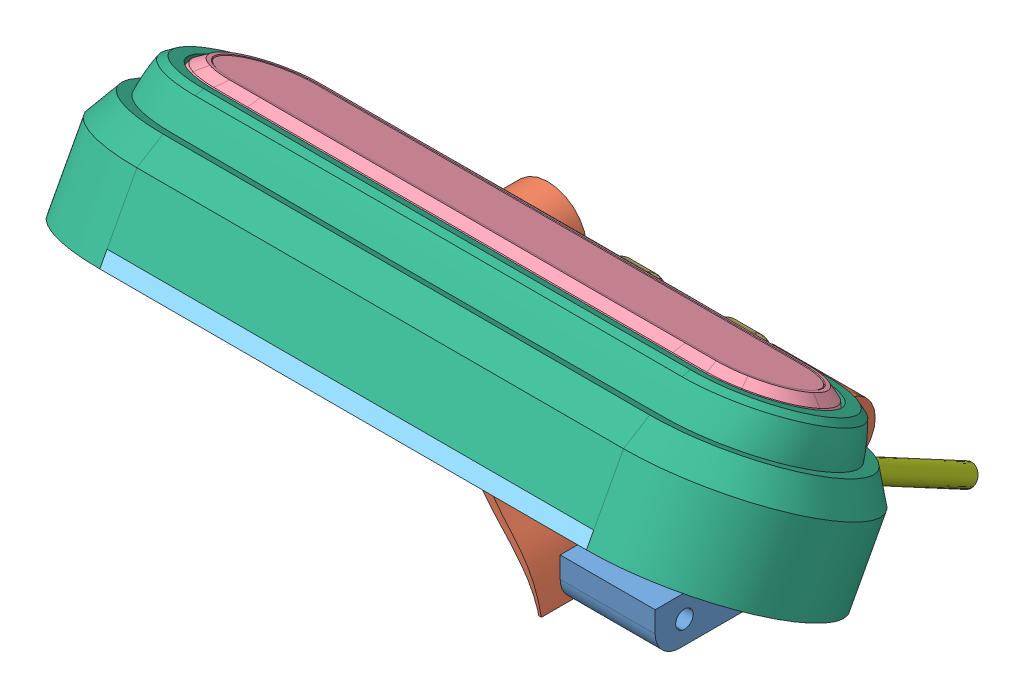
SolidWorks assembly realsense_mount, configuration Default. Lengths in mm.
Overall size (141.5 99.34 86.29).
8 component instances, 7 part files, 15 mates.
Components (placement in the parent):
- camera_mount_clamp-1: camera_mount_clamp [Default] at (0 -14.2875 0) x (0 0 1) z (-1 0 0)
- bike_clamp_pin-1: bike_clamp_pin [Default] at (1.038 25.4 0) x (0 1 0) z (0 0 1)
- camera_support-1: camera_support [Default] at (0 33.1535 14.4321) x (-1 0 0) z (0 0.880921 -0.473263)
- Intel_RealSense_D455-1: Intel_RealSense_D455 [Default] at (0 59.7542 30.1383) x (-1 0 0) z (0 0.880921 -0.473263) size (141.5 46.5 29.01)
  - Intel Realsense D455-1: Intel Realsense D455 [Default] at origin
  - Blocco D455-1: Blocco D455 [Default] at (0 0 -29) x (0 -1 0) z (0 0 1)
  - Cover Telecamera-1: Cover Telecamera [Default] at (0 0 -1.5) x (0 -1 0) z (0 0 1)
- USB C amazon basic-1: USB C amazon basic [Default] at (37.01 26.8658 17.4242) x (0 -0.473263 -0.880921) z (1 0 0)
Mates (geometry in assembly coordinates):
- Coincident1: coordinate: point of camera_mount-1
- Coincident2: coincident anti-aligned: plane of camera_mount_clamp-1 through (0 -14.2875 0) normal (-1 0 0)
- Concentric1: concentric anti-aligned: cylinder of camera_mount-1 through (12.954 -14.2875 6.985) axis (1 0 0) radius 2.4574; cylinder of camera_mount_clamp-1 through (-9.271 -14.2875 6.985) axis (-1 0 0) radius 1.7272
- Parallel1: parallel aligned: plane of camera_mount-1 through (-9.779 -19.05 12.7) normal (0 -1 0); plane of camera_mount_clamp-1 through (0 -18.7325 0) normal (0 -1 0)
- Concentric2: concentric anti-aligned: cylinder of camera_mount-1 through (-6.604 25.4 0) axis (-1 0 0) radius 3.5; cylinder of bike_clamp_pin-1 through (-31.462 25.4 0) axis (1 0 0) radius 3
- Parallel2: parallel aligned: plane of bike_clamp_pin-1 through (1.038 25.4 0) normal (0 0 1)
- Concentric4: concentric aligned: cylinder of bike_clamp_pin-1 through (-31.462 25.4 0) axis (1 0 0) radius 3; cylinder of camera_support-1 through (13.462 25.4 0) axis (1 0 0) radius 3
- Coincident10: coincident anti-aligned: plane of camera_support-1 through (0 33.1535 14.4321) normal (-1 0 0)
- Concentric5: concentric anti-aligned: cylinder of camera_support-1 through (0 34.6561 17.2291) axis (0 0.473263 0.880921) radius 3.5712; cylinder of Intel_RealSense_D455-1/Cover Telecamera-1 through (0 34.6561 17.2291) axis (0 -0.473263 -0.880921) radius 4.365
- Coincident11: coincident anti-aligned: plane of camera_support-1 through (0 34.6561 17.2291) normal (0 0.473263 0.880921); plane of Intel_RealSense_D455-1/Cover Telecamera-1 through (-47.5 23.2041 23.3815) normal (0 -0.473263 -0.880921)
- Parallel5: parallel aligned: plane of camera_support-1 through (-7.0995 29.0622 20.2343) normal (0 -0.880921 0.473263); plane of Intel_RealSense_D455-1/Blocco D455-1 through (47.5 34.2075 43.8629) normal (0 -0.880921 0.473263)
- Coincident13: coincident anti-aligned: plane of Intel_RealSense_D455-1/Intel Realsense D455-1 through (37.01 38.988 30.6382) normal (0 -0.880921 0.473263); plane of USB C amazon basic-1 through (41.16 35.8585 24.8131) normal (0 0.880921 -0.473263)
- Coincident14: coincident anti-aligned: plane of Intel_RealSense_D455-1/Intel Realsense D455-1 through (37.01 37.9645 31.6279) normal (0 -0.473263 -0.880921); plane of USB C amazon basic-1 through (37.01 38.1363 31.5356) normal (0 0.473263 0.880921)
- Coincident15: coincident aligned: plane of Intel_RealSense_D455-1/Intel Realsense D455-1 through (37.01 59.7542 30.1383) normal (1 0 0); plane of USB C amazon basic-1 through (37.01 26.8658 17.4242) normal (1 0 0)
- Distance2: distance = 3.5 mm anti-aligned: plane of camera_support-1 through (-13.462 29.0622 20.2343) normal (-1 0 0); plane of bike_clamp_pin-1 through (-16.962 25.4 0) normal (1 0 0)
